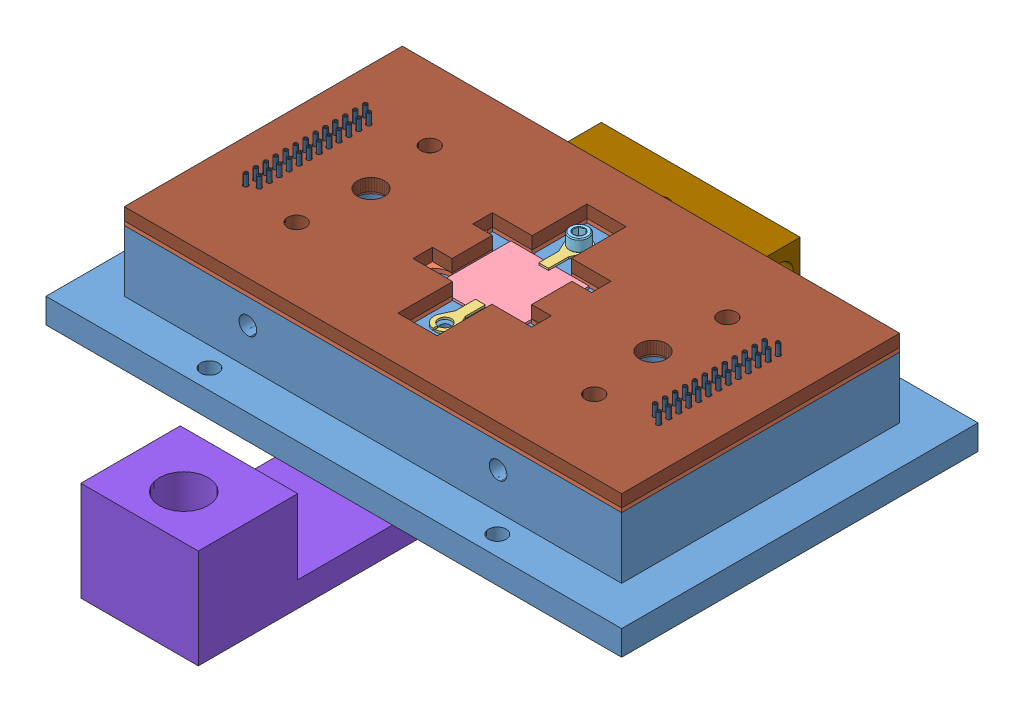
SolidWorks assembly Copper_spce_assembly, configuration Default. Lengths in mm.
Overall size (73.5 19.15 71.66).
22 component instances, 14 part files, 37 mates.
Components (placement in the parent):
- Lid_nopocket-1: Lid_nopocket [Default] at (-5.3766 55.1618 62.3147) size (73.5 11 45.5)
- Sheet_Space-1: Sheet_Space [Default] at (31.3734 66.1618 85.0647) size (63.5 0.51 35.5)
- BeCu_Clamp-1: BeCu_Clamp [Default] at (31.3734 66.7158 76.5031) x (-1 0 0) z (0 0 1) size (2.82 0.25 5.93)
- example_chip-1: example_chip [Default] at (36.2984 66.4618 80.1397) x (-1 0 0) z (0 0 1) size (10 0.3 10)
- BeCu_Clamp-2: BeCu_Clamp [Default] at (31.3734 66.4618 93.6263) x (-1 0 0) z (0 0 -1) size (2.82 0.25 5.93)
- 92196A047_18-8 Stainless Steel Socket Head Screw-2: 92196A047_18-8 Stainless Steel Socket Head Screw [92196A047] at (31.3734 66.684 76.5031) x (0.977938 0 0.208893) z (0 1 0) size (2.44 2.44 3.27)
- 380-025-213L001.step-1: 380-025-213L001.step [Default] at (1.8784 61.2698 85.0647) x (0 0 -1) z (0 1 0) size (29.7 7.35 10.8)
- PCB_TES_Assem-1: PCB_TES_Assem [Default] at (-36.9478 115.625 46.8037) x (0 0 1) z (1 0 0) size (32 13.01 62) (hidden)
  - Micro_D_TES_Array_Model-1: Micro_D_TES_Array_Model [Default] at (22.261 48.1552 37.3212) size (32 0.8 62)
  - 380-025-113L001.step-1: 380-025-113L001.step [Default] at (38.261 58.9552 97.8162) x (-1 0 0) z (0 1 0) size (29.7 7.35 13.01)
  - 380-025-113L001.step-2: 380-025-113L001.step [Default] at (38.261 58.9552 38.8262) x (1 0 0) z (0 1 0) size (29.7 7.35 13.01)
- Box02_Uni-1: Box02_Uni [Default] at (31.3734 58.3368 62.3147) size (38.34 25.18 45.5) (hidden)
- Box02_Uni-2: Box02_Uni [Default] at (31.3734 58.3368 107.8147) x (-1 0 0) z (0 0 -1) size (38.34 25.18 45.5) (hidden)
- Bottom_Block_off_plate-1: Bottom_Block_off_plate [Default] at (10.3734 55.1618 91.0647) x (1 0 0) z (0 0 -1) size (42 3.22 12)
- example_cold_mount-1: example_cold_mount [Default] at (38.8734 51.9868 132.6209) x (-1 0 0) z (0 0 -1) size (15 12.7 40.72)
- Heater_Cart_02-1: Heater_Cart_02 [Default] at (44.0734 66.1618 67.3147) x (-1 0 0) z (0 0 -1) size (38.1 6.35 6.35)
- micro-d-tes-aaray.step-1: micro-d-tes-aaray.step [Default] at (-0.3766 66.6698 102.8147) x (0 0 -1) z (0 1 0) size (35.5 63.5 13.01)
  - 380-025-113L001.step-1: 380-025-113L001.step [Default] at (17.75 -2.2745 -10.05) x (-1 0 0) z (0 0 -1) size (29.7 7.35 13.01)
    - SOLID.step-1: SOLID.step [Default] at origin size (29.7 7.35 13.01)
  - 380-025-113L001.step-2: 380-025-113L001.step [Default] at (17.75 -61.2245 -10.05) x (1 0 0) z (0 0 -1) size (29.7 7.35 13.01)
    - SOLID.step-1: SOLID.step [Default] at origin size (29.7 7.35 13.01)
  - _autosave-micro-d-tes-aaray PCB.step-1: _autosave-micro-d-tes-aaray PCB.step [Default] at origin size (35.5 63.5 1.58)
Mates (geometry in assembly coordinates):
- Coincident3: coincident anti-aligned: plane of Lid_nopocket-1 through (-5.3766 66.1618 62.3147) normal (0 1 0); plane of example_chip-1 through (36.2984 66.1618 80.1397) normal (0 -1 0)
- Coincident6: coincident anti-aligned: plane of BeCu_Clamp-1 through (31.3734 66.4618 76.5031) normal (0 -1 0); plane of example_chip-1 through (36.2984 66.4618 80.1397) normal (0 1 0)
- Concentric6: concentric anti-aligned: cylinder of Lid_nopocket-1 through (31.3734 66.1618 76.5031) axis (0 1 0) radius 0.5956; circle of BeCu_Clamp-1
- Coincident7: coincident anti-aligned: plane of example_chip-1 through (36.2984 66.4618 80.1397) normal (0 1 0); plane of BeCu_Clamp-2 through (31.3734 66.4618 93.6263) normal (0 -1 0)
- Concentric7: concentric aligned: cylinder of Lid_nopocket-1 through (31.3734 66.1618 93.6263) axis (0 1 0) radius 0.5956; circle of BeCu_Clamp-2
- Parallel2: parallel anti-aligned: line of BeCu_Clamp-1 through (31.9957 66.7158 78.4843) axis (0 0 1); line of BeCu_Clamp-2 through (31.9957 66.7158 91.6451) axis (0 0 -1)
- Concentric14: concentric aligned: cylinder of Lid_nopocket-1 through (31.3734 66.1618 76.5031) axis (0 1 0) radius 0.5956; circle of 92196A047_18-8 Stainless Steel Socket Head Screw-2
- Coincident15: coincident anti-aligned: plane of BeCu_Clamp-1 through (31.3734 66.7158 76.5031) normal (0 1 0); plane of 92196A047_18-8 Stainless Steel Socket Head Screw-2 through (31.6281 66.7158 75.3108) normal (0 -1 0)
- Coincident21: coincident: cylinder of Lid_nopocket-1 through (13.3734 58.3368 85.0647) axis (0 -1 0) radius 2.2479; circle of PCB_TES_Assem-1/Micro_D_TES_Array_Model-1
- Coincident22: coincident: cylinder of Lid_nopocket-1 through (49.3734 58.3368 85.0647) axis (0 -1 0) radius 2.2479; circle of PCB_TES_Assem-1/Micro_D_TES_Array_Model-1
- Coincident24: coincident anti-aligned: plane of Lid_nopocket-1 through (-5.3766 66.1618 62.3147) normal (0 1 0); plane of Sheet_Space-1 through (31.3734 66.1618 85.0647) normal (0 -1 0)
- Concentric23: concentric anti-aligned: cylinder of Sheet_Space-1 through (49.3734 66.6698 85.0647) axis (0 -1 0) radius 2.1446; cylinder of PCB_TES_Assem-1/Micro_D_TES_Array_Model-1 through (49.3734 66.6698 85.0647) axis (0 1 0) radius 2.1526
- Concentric24: concentric anti-aligned: cylinder of Sheet_Space-1 through (13.3734 66.6698 85.0647) axis (0 -1 0) radius 2.1446; cylinder of PCB_TES_Assem-1/Micro_D_TES_Array_Model-1 through (13.3734 66.6698 85.0647) axis (0 1 0) radius 2.1526
- Coincident25: coincident anti-aligned: plane of Sheet_Space-1 through (31.3734 66.6698 85.0647) normal (0 1 0); plane of PCB_TES_Assem-1/Micro_D_TES_Array_Model-1 through (0.3734 66.6698 69.0647) normal (0 -1 0)
- Coincident26: coincident anti-aligned: plane of Sheet_Space-1 through (31.3734 66.6698 90.1397) normal (0 0 -1); plane of example_chip-1 through (36.2984 66.1618 90.1397) normal (0 0 1)
- Coincident27: coincident anti-aligned: plane of Sheet_Space-1 through (26.2984 66.6698 85.0647) normal (1 0 0); plane of example_chip-1 through (26.2984 66.1618 80.1397) normal (-1 0 0)
- Concentric25: concentric aligned: cylinder of 380-025-213L001.step-1 through (5.0034 59.8693 77.4447) axis (0 -1 0) radius 0.285; cylinder of PCB_TES_Assem-1/380-025-113L001.step-2 through (5.0034 60.3698 77.4447) axis (0 -1 0) radius 0.475
- Concentric26: concentric aligned: cylinder of 380-025-213L001.step-1 through (5.0034 59.8693 92.6847) axis (0 -1 0) radius 0.285; cylinder of PCB_TES_Assem-1/380-025-113L001.step-2 through (5.0034 60.3698 92.6847) axis (0 -1 0) radius 0.475
- Coincident29: coincident anti-aligned: plane of 380-025-213L001.step-1 through (8.2626 61.2698 95.106) normal (0 1 0); plane of PCB_TES_Assem-1/380-025-113L001.step-2 through (9.2194 61.2698 69.7767) normal (0 -1 0)
- Concentric27: concentric aligned: cylinder of Lid_nopocket-1 through (12.9984 55.1618 64.8147) axis (0 -1 0) radius 1.1303; cylinder of Box02_Uni-1 through (12.9984 58.3368 64.8147) axis (0 -1 0) radius 0.889
- Concentric28: concentric aligned: cylinder of Lid_nopocket-1 through (12.9984 55.1618 105.3147) axis (0 -1 0) radius 1.1303; circle of Box02_Uni-1
- Coincident30: coincident anti-aligned: plane of Lid_nopocket-1 through (-5.3766 58.3368 62.3147) normal (0 1 0); plane of Box02_Uni-1 through (31.3734 58.3368 62.3147) normal (0 -1 0)
- Concentric29: concentric aligned: cylinder of Lid_nopocket-1 through (49.7484 55.1618 64.8147) axis (0 -1 0) radius 1.1303; cylinder of Box02_Uni-2 through (49.7484 58.3368 64.8147) axis (0 -1 0) radius 0.889
- Concentric30: concentric aligned: cylinder of Lid_nopocket-1 through (49.7484 55.1618 105.3147) axis (0 -1 0) radius 1.1303; cylinder of Box02_Uni-2 through (49.7484 58.3368 105.3147) axis (0 -1 0) radius 0.889
- Coincident31: coincident anti-aligned: plane of Lid_nopocket-1 through (-5.3766 58.3368 62.3147) normal (0 1 0); plane of Box02_Uni-2 through (31.3734 58.3368 107.8147) normal (0 -1 0)
- Concentric31: concentric aligned: circle of Lid_nopocket-1; circle of Bottom_Block_off_plate-1
- Concentric32: concentric aligned: circle of Lid_nopocket-1; circle of Bottom_Block_off_plate-1
- Coincident32: coincident anti-aligned: plane of Lid_nopocket-1 through (-5.3766 55.1618 62.3147) normal (0 -1 0); plane of Bottom_Block_off_plate-1 through (10.3734 55.1618 91.0647) normal (0 1 0)
- Concentric35: concentric anti-aligned: cylinder of Lid_nopocket-1 through (27.5634 55.1618 93.6947) axis (0 -1 0) radius 0.889; circle of example_cold_mount-1
- Coincident34: coincident anti-aligned: plane of Lid_nopocket-1 through (-5.3766 55.1618 62.3147) normal (0 -1 0); plane of example_cold_mount-1 through (38.8734 55.1618 132.6209) normal (0 1 0)
- Concentric36: concentric aligned: cylinder of Lid_nopocket-1 through (35.1834 55.1618 93.6947) axis (0 -1 0) radius 0.889; cylinder of example_cold_mount-1 through (35.1834 55.1618 93.6947) axis (0 -1 0) radius 0.889
- Concentric38: concentric aligned: cylinder of Lid_nopocket-1 through (47.3484 62.9868 67.3147) axis (0 0 -1) radius 1.1303; circle of Heater_Cart_02-1
- Concentric39: concentric anti-aligned: cylinder of Lid_nopocket-1 through (15.3984 62.9868 67.3147) axis (0 0 -1) radius 1.1303; cylinder of Heater_Cart_02-1 through (15.3984 62.9868 66.3147) axis (0 0 1) radius 1.4732
- Coincident35: coincident anti-aligned: plane of Lid_nopocket-1 through (-5.3766 66.1618 67.3147) normal (0 0 -1); plane of Heater_Cart_02-1 through (44.0734 66.1618 67.3147) normal (0 0 1)
- Concentric40: concentric aligned: cylinder of Lid_nopocket-1 through (12.3734 66.1618 76.5647) axis (0 1 0) radius 0.889; cylinder of micro-d-tes-aaray.step-1/_autosave-micro-d-tes-aaray PCB.step-1 through (12.3734 65.8798 76.5647) axis (0 1 0) radius 1.15
- Concentric41: concentric aligned: cylinder of Lid_nopocket-1 through (12.3734 66.1618 93.5647) axis (0 1 0) radius 0.889; cylinder of micro-d-tes-aaray.step-1/_autosave-micro-d-tes-aaray PCB.step-1 through (12.3734 65.8798 93.5647) axis (0 1 0) radius 1.15
- Coincident36: coincident anti-aligned: plane of Sheet_Space-1 through (31.3734 66.6698 85.0647) normal (0 1 0); plane of micro-d-tes-aaray.step-1/_autosave-micro-d-tes-aaray PCB.step-1 through (31.3734 66.6698 85.0647) normal (0 -1 0)
